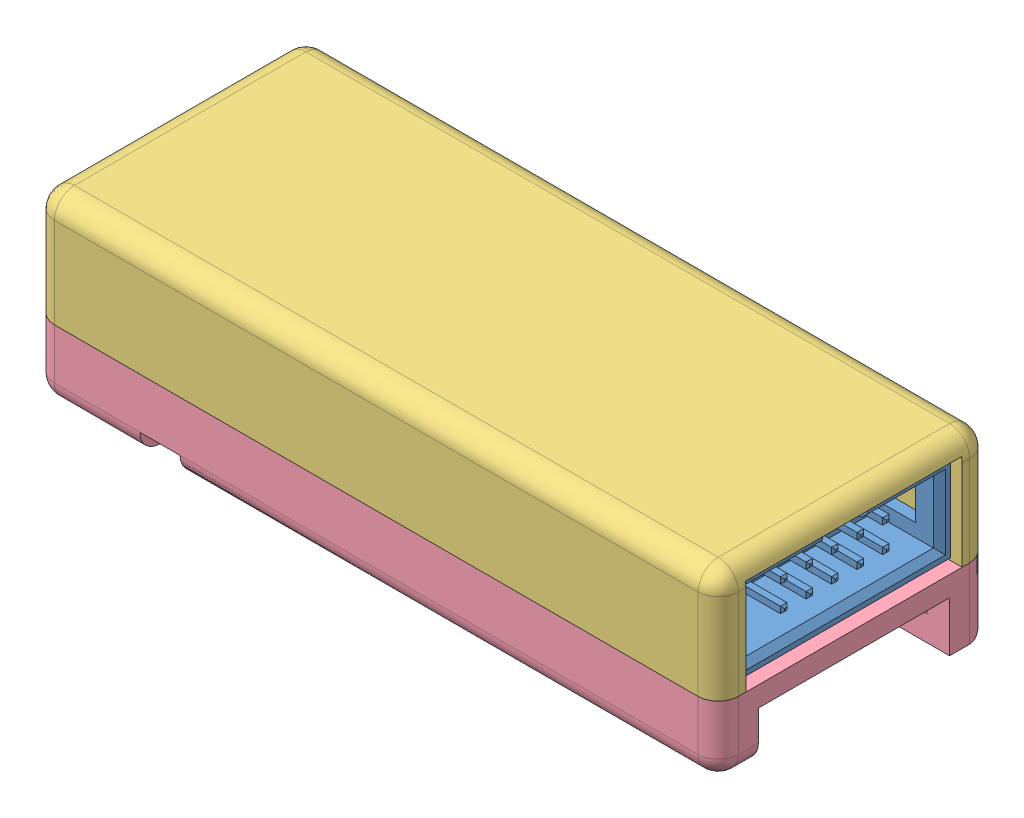
SolidWorks assembly Сборка J-Link Isolated_FFC, configuration По умолчанию. Lengths in mm.
Overall size (68 18.11 27).
6 component instances, 5 part files, 9 mates.
Components (placement in the parent):
- Board-1: Board [По умолчанию] at (-31.5 6.9786 0) x (0 0 1) z (0 1 0) size (22 66.22 13.13)
- M2X10MM_HEXAGON-1: M2X10MM_HEXAGON [M2X10mm] at (-21.5 0 9) x (0 0 -1) z (0 -1 0) size (3.8 3.8 12.11)
- M2X10MM_HEXAGON-2: M2X10MM_HEXAGON [M2X10mm] at (-21.5 0 -9) x (0 0 -1) z (0 -1 0) size (3.8 3.8 12.11)
- Деталь4^Сборка J-Link Isolated_FFC-1: Деталь4^Сборка J-Link Isolated_FFC [По умолчанию] at origin (virtual)
- Top-1: Top [По умолчанию] at (0 7 0) size (68 11 27)
- Bottom_FFC-1: Bottom_FFC [По умолчанию] at origin size (68 7 27)
Mates (geometry in assembly coordinates):
- Совпадение1: coincident anti-aligned: plane of Bottom-1 through (0 5.4 0) normal (0 1 0); plane of Board-1 through (-30.5 5.4 -11) normal (0 -1 0)
- Концентричный2: concentric aligned: cylinder of Bottom-1 through (23 8.6919 -11) axis (0 -1 0) radius 0.7; cylinder of Board-1 through (23 5.4 -11) axis (0 -1 0) radius 0.75
- Концентричный4: concentric anti-aligned: cylinder of Bottom-1 through (-21.5 0 9) axis (0 1 0) radius 1.1; cylinder of M2X10MM_HEXAGON-1 through (-21.5 0 9) axis (0 -1 0) radius 1
- Совпадение3: coincident anti-aligned: plane of Bottom-1 through (-21.5 2 9) normal (0 -1 0); plane of M2X10MM_HEXAGON-1 through (-19.76 2 9) normal (0 1 0)
- Концентричный5: concentric anti-aligned: cylinder of Bottom-1 through (-21.5 0 -9) axis (0 1 0) radius 1.1; cylinder of M2X10MM_HEXAGON-2 through (-21.5 0 -9) axis (0 -1 0) radius 1
- Совпадение4: coincident anti-aligned: plane of Bottom-1 through (-21.5 2 -9) normal (0 -1 0); plane of M2X10MM_HEXAGON-2 through (-19.76 2 -9) normal (0 1 0)
- Совпадение5: coincident anti-aligned: plane of Bottom-1 through (0 7 0) normal (0 1 0); plane of Top-1 through (0 7 0) normal (0 -1 0)
- Совпадение6: coincident anti-aligned: plane of Top-1 through (0 7 0) normal (0 -1 0); plane of Bottom_FFC-1 through (0 7 0) normal (0 1 0)
- Концентричный7: concentric anti-aligned: circle of Top-1; circle of Bottom_FFC-1
